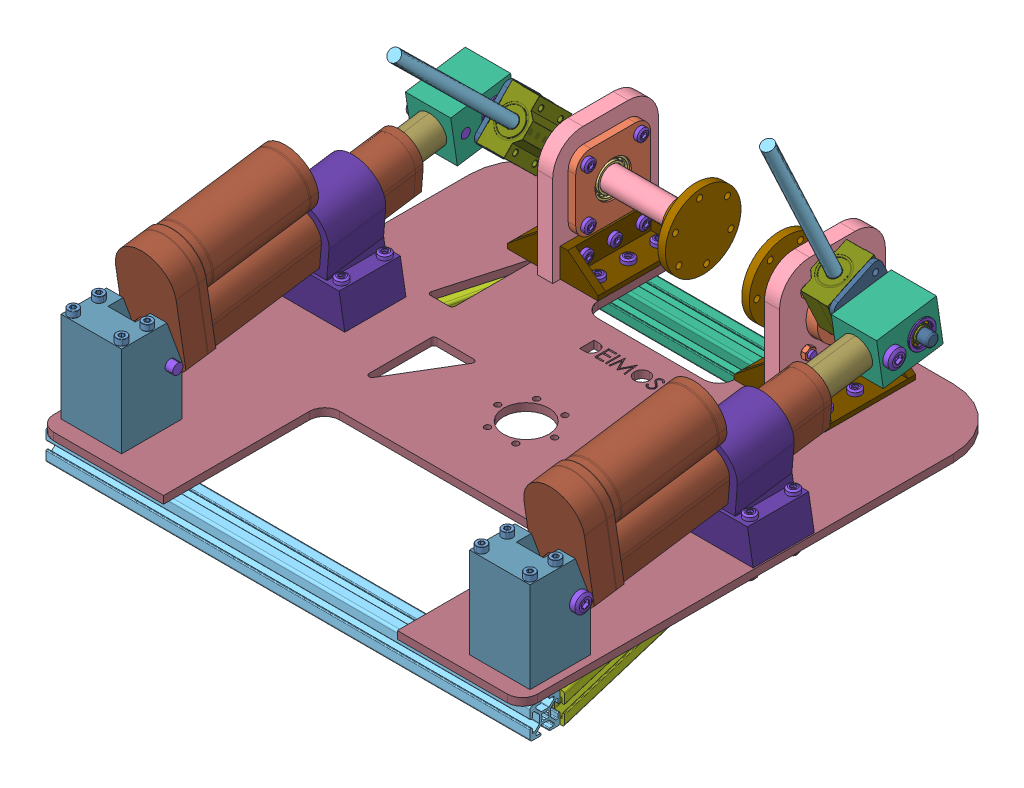
SolidWorks assembly Arm_base_2025_Final, configuration Default. Lengths in mm. (continued)
Mates (geometry in assembly coordinates): (continued)
- Distance14: distance = 6 mm anti-aligned: plane of V8_bearing and cam connection_for_v4URC 2024_V4 laser cut-2 through (396.4714 168.2112 182.1724) normal (1 0 0); plane of Connector to Linear bearing-2/V8_F688ZZ_assemblyURC 2024_V4-2/V8_F688ZZ_HousingURC 2024_V4-1 through (402.4714 162.026 159.969) normal (-1 0 0)
- Distance16: distance = 6 mm anti-aligned: plane of V8_bearing and cam connection_for_v4URC 2024_V4 laser cut-1 through (170.6714 137.31 173.1714) normal (-1 0 0); plane of Connector to Linear bearing-1/V8_F688ZZ_assemblyURC 2024_V4-1/V8_F688ZZ_HousingURC 2024_V4-1 through (164.6714 160.303 171.5672) normal (1 0 0)
- Coincident76: coincident anti-aligned: plane of base bearing assambly-1/base shaft bearing housing-1 through (213.5714 172.6403 148.5796) normal (-1 0 0); plane of V8_bearing holder holderURC 2024_V4-1 through (213.5714 172.6403 113.5796) normal (1 0 0)
- Concentric84: concentric anti-aligned: cylinder of base bearing assambly-1/base shaft bearing housing-1 through (208.5714 155.1403 166.0796) axis (1 0 0) radius 2; cylinder of V8_bearing holder holderURC 2024_V4-1 through (213.5714 155.1403 166.0796) axis (-1 0 0) radius 2
- Concentric91: concentric aligned: cylinder of LA_back holder-2 through (402.5714 180.6403 419.5796) axis (0 -1 0) radius 2; cylinder of Screw_DIN_912_M4x70_A2.step-1 through (402.5714 102.6403 419.5796) axis (0 -1 0) radius 2
- Coincident83: coincident anti-aligned: plane of LA_back holder-2 through (418.5714 152.6403 403.5796) normal (0 1 0); plane of Screw_DIN_912_M4x70_A2.step-1 through (402.5714 152.6403 419.5796) normal (0 -1 0)
- Concentric92: concentric aligned: cylinder of LA_back holder-2 through (434.5714 180.6403 419.5796) axis (0 -1 0) radius 2; cylinder of Screw_DIN_912_M4x70_A2.step-2 through (434.5714 102.6403 419.5796) axis (0 -1 0) radius 2
- Coincident84: coincident anti-aligned: plane of LA_back holder-2 through (418.5714 152.6403 403.5796) normal (0 1 0); plane of Screw_DIN_912_M4x70_A2.step-2 through (434.5714 152.6403 419.5796) normal (0 -1 0)
- Concentric93: concentric aligned: cylinder of LA_back holder-2 through (434.5714 180.6403 402.6026) axis (0 -1 0) radius 2; cylinder of Screw_DIN_912_M4x70_A2.step-4 through (434.5714 102.6403 402.6026) axis (0 -1 0) radius 2
- Coincident85: coincident anti-aligned: plane of LA_back holder-2 through (418.5714 152.6403 403.5796) normal (0 1 0); plane of Screw_DIN_912_M4x70_A2.step-4 through (434.5714 152.6403 402.6026) normal (0 -1 0)
- Concentric94: concentric aligned: cylinder of LA_back holder-2 through (402.5714 180.6403 402.6026) axis (0 -1 0) radius 2; cylinder of Screw_DIN_912_M4x70_A2.step-6 through (402.5714 102.6403 402.6026) axis (0 -1 0) radius 2
- Coincident86: coincident anti-aligned: plane of LA_back holder-2 through (418.5714 152.6403 403.5796) normal (0 1 0); plane of Screw_DIN_912_M4x70_A2.step-6 through (402.5714 152.6403 402.6026) normal (0 -1 0)
- Concentric95: concentric aligned: cylinder of LA_back holder-1 through (164.5714 180.6403 419.5796) axis (0 -1 0) radius 2; cylinder of Screw_DIN_912_M4x70_A2.step-8 through (164.5714 102.6403 419.5796) axis (0 -1 0) radius 2
- Coincident87: coincident anti-aligned: plane of LA_back holder-1 through (148.5714 152.6403 403.5796) normal (0 1 0); plane of Screw_DIN_912_M4x70_A2.step-8 through (164.5714 152.6403 419.5796) normal (0 -1 0)
- Concentric96: concentric aligned: cylinder of LA_back holder-1 through (164.5714 180.6403 402.6026) axis (0 -1 0) radius 2; cylinder of Screw_DIN_912_M4x70_A2.step-10 through (164.5714 102.6403 402.6026) axis (0 -1 0) radius 2
- Coincident88: coincident anti-aligned: plane of LA_back holder-1 through (148.5714 152.6403 403.5796) normal (0 1 0); plane of Screw_DIN_912_M4x70_A2.step-10 through (164.5714 152.6403 402.6026) normal (0 -1 0)
- Concentric97: concentric aligned: cylinder of LA_back holder-1 through (132.5714 180.6403 419.5796) axis (0 -1 0) radius 2; cylinder of Screw_DIN_912_M4x70_A2.step-12 through (132.5714 102.6403 419.5796) axis (0 -1 0) radius 2
- Coincident89: coincident anti-aligned: plane of LA_back holder-1 through (148.5714 152.6403 403.5796) normal (0 1 0); plane of Screw_DIN_912_M4x70_A2.step-12 through (132.5714 152.6403 419.5796) normal (0 -1 0)
- Concentric98: concentric aligned: cylinder of LA_back holder-1 through (132.5714 180.6403 402.6026) axis (0 -1 0) radius 2; cylinder of Screw_DIN_912_M4x70_A2.step-14 through (132.5714 102.6403 402.6026) axis (0 -1 0) radius 2
- Coincident90: coincident anti-aligned: plane of LA_back holder-1 through (148.5714 152.6403 403.5796) normal (0 1 0); plane of Screw_DIN_912_M4x70_A2.step-14 through (132.5714 152.6403 402.6026) normal (0 -1 0)
- Concentric99: concentric anti-aligned: cylinder of V8_base plate for LAURC 2024_V4-1 through (402.5714 82.6403 419.5796) axis (0 1 0) radius 2; cylinder of hex nut style 1 gradeab_iso-8 through (402.5714 87.6403 419.5796) axis (0 -1 0) radius 1.65
- Coincident91: coincident anti-aligned: plane of V8_base plate for LAURC 2024_V4-1 through (283.5714 87.6403 412.2334) normal (0 -1 0); plane of hex nut style 1 gradeab_iso-8 through (395.5728 87.6403 419.4444) normal (0 1 0)
- Concentric100: concentric anti-aligned: cylinder of V8_base plate for LAURC 2024_V4-1 through (434.5714 82.6403 419.5796) axis (0 1 0) radius 2; cylinder of hex nut style 1 gradeab_iso-9 through (434.5714 87.6403 419.5796) axis (0 -1 0) radius 1.65
- Coincident92: coincident anti-aligned: plane of V8_base plate for LAURC 2024_V4-1 through (283.5714 87.6403 412.2334) normal (0 -1 0); plane of hex nut style 1 gradeab_iso-9 through (427.6727 87.6403 420.7658) normal (0 1 0)
- Concentric101: concentric aligned: circle of Screw_DIN_912_M4x70_A2.step-4; cylinder of hex nut style 1 gradeab_iso-11 through (434.5714 87.6403 402.6026) axis (0 -1 0) radius 1.65
- Coincident93: coincident anti-aligned: plane of V8_base plate for LAURC 2024_V4-1 through (283.5714 87.6403 412.2334) normal (0 -1 0); plane of hex nut style 1 gradeab_iso-11 through (430.6304 87.6403 408.3878) normal (0 1 0)
- Concentric102: concentric aligned: cylinder of Screw_DIN_912_M4x70_A2.step-6; cylinder of hex nut style 1 gradeab_iso-14 through (402.5714 87.6403 402.6026) axis (0 -1 0) radius 1.65
- Coincident94: coincident anti-aligned: plane of V8_base plate for LAURC 2024_V4-1 through (283.5714 87.6403 412.2334) normal (0 -1 0); plane of hex nut style 1 gradeab_iso-14 through (398.6304 87.6403 408.3878) normal (0 1 0)
- Concentric103: concentric anti-aligned: cylinder of V8_base plate for LAURC 2024_V4-1; cylinder of hex nut style 1 gradeab_iso-16 through (164.5714 87.6403 419.5796) axis (0 -1 0) radius 1.65
- Coincident95: coincident anti-aligned: plane of V8_base plate for LAURC 2024_V4-1 through (283.5714 87.6403 412.2334) normal (0 -1 0); plane of hex nut style 1 gradeab_iso-16 through (160.0326 87.6403 424.9087) normal (0 1 0)
- Concentric104: concentric aligned: cylinder of Screw_DIN_912_M4x70_A2.step-10; cylinder of hex nut style 1 gradeab_iso-18 through (164.5714 87.6403 402.6026) axis (0 -1 0) radius 1.65
- Coincident96: coincident anti-aligned: plane of V8_base plate for LAURC 2024_V4-1 through (283.5714 87.6403 412.2334) normal (0 -1 0); plane of hex nut style 1 gradeab_iso-18 through (160.6304 87.6403 408.3878) normal (0 1 0)
- Concentric105: concentric aligned: cylinder of Screw_DIN_912_M4x70_A2.step-12; cylinder of hex nut style 1 gradeab_iso-20 through (132.5714 87.6403 419.5796) axis (0 -1 0) radius 1.65
- Coincident97: coincident anti-aligned: plane of V8_base plate for LAURC 2024_V4-1 through (283.5714 87.6403 412.2334) normal (0 -1 0); plane of hex nut style 1 gradeab_iso-20 through (128.6304 87.6403 425.3648) normal (0 1 0)
- Concentric106: concentric aligned: cylinder of Screw_DIN_912_M4x70_A2.step-14; cylinder of hex nut style 1 gradeab_iso-22 through (132.5714 87.6403 402.6026) axis (0 -1 0) radius 1.65
- Coincident98: coincident anti-aligned: plane of V8_base plate for LAURC 2024_V4-1 through (283.5714 87.6403 412.2334) normal (0 -1 0); plane of hex nut style 1 gradeab_iso-22 through (128.6304 87.6403 408.3878) normal (0 1 0)
- Concentric107: concentric aligned: unknown of linnear rod coupler-2; unknown of lock_nut_for coupler-2
- Concentric108: concentric aligned: cylinder of lock_nut_for coupler-2; cylinder of base bearing assambly-2/base shaft bearing housing-1 through (370.5714 137.6403 148.5796) axis (1 0 0) radius 8
- Coincident100: coincident anti-aligned: plane of V8_base plate for LAURC 2024_V4-1 through (283.5714 92.6403 412.2334) normal (0 1 0); plane of linear_acutator_holder-1 through (394.6971 92.6403 239.7077) normal (0 -1 0)
- Tangent2: tangent: cylinder of linnear rod coupler-2 through (388.2714 137.6403 148.5796) axis (-1 0 0) radius 6; unknown of linear guid rod-2
- Tangent3: tangent: cylinder of linnear rod coupler-1 through (178.8714 137.6403 148.5796) axis (1 0 0) radius 6; unknown of linear guid rod-1
- Concentric109: concentric anti-aligned: cylinder of linnear rod coupler-1 through (178.8714 137.6403 148.5796) axis (1 0 0) radius 6; cylinder of base bearing assambly-1/base shaft bearing housing-1 through (196.5714 137.6403 148.5796) axis (-1 0 0) radius 8
- Concentric110: concentric anti-aligned: cylinder of base bearing assambly-2/base shaft bearing housing-1 through (370.5714 137.6403 148.5796) axis (1 0 0) radius 8; cylinder of V8_shaftURC 2024_V4 real part-1 through (333.5714 137.6403 148.5796) axis (-1 0 0) radius 7.5
- Concentric111: concentric anti-aligned: cylinder of base bearing assambly-1/base shaft bearing housing-1 through (196.5714 137.6403 148.5796) axis (-1 0 0) radius 8; cylinder of V8_shaftURC 2024_V4-1 through (273.0714 137.6403 148.5796) axis (1 0 0) radius 7.5
- Coincident102: coincident aligned: plane of V8_bearing holder holderURC 2024_V4-1 through (203.5714 172.6403 113.5796) normal (0 0 -1); plane of V8_bearing holder holderURC 2024_V4-2 through (363.5714 172.6403 113.5796) normal (0 0 -1)
- Coincident105: coincident aligned: plane of linnear rod coupler-1 through (170.8714 137.6403 148.5796) normal (-1 0 0); plane of V8_shaftURC 2024_V4-1 through (170.8714 137.6403 148.5796) normal (-1 0 0)
- Coincident106: coincident anti-aligned: plane of V8_base plate for LAURC 2024_V4-1 through (283.5714 87.6403 412.2334) normal (0 -1 0); plane of 20 20 aluminium extrusion T slot-1 through (443.5714 87.6403 427.0796) normal (0 1 0)
- Coincident107: coincident aligned: plane of V8_base plate for LAURC 2024_V4-1 through (443.5714 92.6403 412.2334) normal (1 0 0); plane of 20 20 aluminium extrusion T slot-1 through (443.5714 74.5023 409.0876) normal (1 0 0)
- Distance17: distance = 5 mm aligned: plane of 20 20 aluminium extrusion T slot-1 through (443.5714 69.1403 428.5796) normal (0 0 1); plane of V8_base plate for LAURC 2024_V4-1 through (283.5714 92.6403 433.5796) normal (0 0 1)
- Coincident108: coincident anti-aligned: plane of V8_base plate for LAURC 2024_V4-1 through (283.5714 87.6403 412.2334) normal (0 -1 0); plane of 20 20 aluminium extrusion T slot 200 mm-1 through (383.5714 87.6403 157.0796) normal (0 1 0)
- Parallel18: parallel aligned: plane of V8_base plate for LAURC 2024_V4-1 through (443.5714 92.6403 412.2334) normal (1 0 0); plane of 20 20 aluminium extrusion T slot 200 mm-1 through (383.5714 74.5023 139.0876) normal (1 0 0)
- Coincident109: coincident anti-aligned: plane of V8_base plate for LAURC 2024_V4-1 through (283.5714 87.6403 412.2334) normal (0 -1 0); plane of 20 20 aluminium extrusion T slot at angle-1 through (383.9984 87.6403 154.2734) normal (0 1 0)
- Distance18: distance = 60 mm aligned: plane of V8_base plate for LAURC 2024_V4-1 through (443.5714 92.6403 412.2334) normal (1 0 0); plane of 20 20 aluminium extrusion T slot 200 mm-1 through (383.5714 74.5023 139.0876) normal (1 0 0)
- Coincident111: coincident anti-aligned: plane of 20 20 aluminium extrusion T slot 200 mm-1 through (383.5714 69.1403 158.5796) normal (0 0 1); plane of 20 20 aluminium extrusion T slot at angle-1 through (386.5714 87.6403 158.5796) normal (0 0 -1)
- Distance20: distance = 30 mm aligned: plane of V8_base plate for LAURC 2024_V4-1 through (283.5714 92.6403 108.5796) normal (0 0 -1); plane of 20 20 aluminium extrusion T slot 200 mm-1 through (383.5714 86.1403 138.5796) normal (0 0 -1)
- Coincident113: coincident anti-aligned: plane of 20 20 aluminium extrusion T slot 200 mm-1 through (383.5714 69.1403 158.5796) normal (0 0 1); plane of 20 20 aluminium extrusion T slot at angle-2 through (201.1363 67.6403 158.5796) normal (0 0 -1)
- Parallel19: parallel anti-aligned: plane of 20 20 aluminium extrusion T slot-1 through (443.5714 74.5023 408.5796) normal (0 0 -1); plane of 20 20 aluminium extrusion T slot at angle-2 through (141.3123 67.6403 408.5333) normal (0 0 1)
- Coincident115: coincident anti-aligned: plane of V8_base plate for LAURC 2024_V4-1 through (283.5714 87.6403 412.2334) normal (0 -1 0); plane of 20 20 aluminium extrusion T slot at angle-2 through (122.2062 87.6403 408.8825) normal (0 1 0)
- Distance21: distance = 3 mm aligned: line of 20 20 aluminium extrusion T slot at angle-2 through (180.5714 69.1403 158.5796) axis (0 1 0); line of 20 20 aluminium extrusion T slot 200 mm-1 through (183.5714 69.1403 158.5796) axis (0 1 0)
- Lock1: lock: 
- Concentric112: concentric anti-aligned: cylinder of l bracket_arm base flang-1 through (378.5714 90.6403 168.5796) axis (0 1 0) radius 2; cylinder of hexalobular socket pan head_iso-2 through (378.5714 83.6403 168.5796) axis (0 -1 0) radius 2.35
- Coincident116: coincident anti-aligned: plane of l bracket_arm base flang-1 through (388.5714 95.6403 178.5796) normal (0 1 0); plane of hexalobular socket pan head_iso-2 through (380.9214 95.6403 168.5796) normal (0 -1 0)
- Concentric113: concentric anti-aligned: cylinder of l bracket_arm base flang-1 through (378.5714 90.6403 148.5796) axis (0 1 0) radius 2; cylinder of hexalobular socket pan head_iso-3 through (378.5714 83.6403 148.5796) axis (0 -1 0) radius 2.35
- Coincident117: coincident anti-aligned: plane of l bracket_arm base flang-1 through (388.5714 95.6403 178.5796) normal (0 1 0); plane of hexalobular socket pan head_iso-3 through (380.9214 95.6403 148.5796) normal (0 -1 0)
- Concentric114: concentric anti-aligned: cylinder of l bracket_arm base flang-1 through (378.5714 90.6403 128.5796) axis (0 1 0) radius 2; cylinder of hexalobular socket pan head_iso-4 through (378.5714 83.6403 128.5796) axis (0 -1 0) radius 2.35
- Coincident118: coincident anti-aligned: plane of l bracket_arm base flang-1 through (388.5714 95.6403 178.5796) normal (0 1 0); plane of hexalobular socket pan head_iso-4 through (380.9214 95.6403 128.5796) normal (0 -1 0)
- Concentric115: concentric anti-aligned: cylinder of l bracket_arm base flang-2 through (338.5714 90.6403 168.5796) axis (0 1 0) radius 2; cylinder of hexalobular socket pan head_iso-5 through (338.5714 83.6403 168.5796) axis (0 -1 0) radius 2.35
- Coincident119: coincident anti-aligned: plane of l bracket_arm base flang-2 through (328.5714 95.6403 118.5796) normal (0 1 0); plane of hexalobular socket pan head_iso-5 through (340.9214 95.6403 168.5796) normal (0 -1 0)
- Concentric116: concentric anti-aligned: cylinder of l bracket_arm base flang-2 through (338.5714 90.6403 148.5796) axis (0 1 0) radius 2; cylinder of hexalobular socket pan head_iso-6 through (338.5714 83.6403 148.5796) axis (0 -1 0) radius 2.35
- Coincident120: coincident anti-aligned: plane of l bracket_arm base flang-2 through (328.5714 95.6403 118.5796) normal (0 1 0); plane of hexalobular socket pan head_iso-6 through (340.9214 95.6403 148.5796) normal (0 -1 0)
- Concentric117: concentric anti-aligned: cylinder of l bracket_arm base flang-2 through (338.5714 90.6403 128.5796) axis (0 1 0) radius 2; cylinder of hexalobular socket pan head_iso-7 through (338.5714 83.6403 128.5796) axis (0 -1 0) radius 2.35
- Coincident121: coincident anti-aligned: plane of l bracket_arm base flang-2 through (328.5714 95.6403 118.5796) normal (0 1 0); plane of hexalobular socket pan head_iso-7 through (340.9214 95.6403 128.5796) normal (0 -1 0)
- Concentric118: concentric anti-aligned: cylinder of l bracket_arm base flang-4 through (228.5714 90.6403 128.5796) axis (0 1 0) radius 2; cylinder of hexalobular socket pan head_iso-8 through (228.5714 83.6403 128.5796) axis (0 -1 0) radius 2.35
- Coincident122: coincident anti-aligned: plane of l bracket_arm base flang-4 through (238.5714 95.6403 178.5796) normal (0 1 0); plane of hexalobular socket pan head_iso-8 through (230.9214 95.6403 128.5796) normal (0 -1 0)
- Concentric119: concentric anti-aligned: cylinder of l bracket_arm base flang-4 through (228.5714 90.6403 148.5796) axis (0 1 0) radius 2; cylinder of hexalobular socket pan head_iso-9 through (228.5714 83.6403 148.5796) axis (0 -1 0) radius 2.35
- Coincident123: coincident anti-aligned: plane of l bracket_arm base flang-4 through (238.5714 95.6403 178.5796) normal (0 1 0); plane of hexalobular socket pan head_iso-9 through (230.9214 95.6403 148.5796) normal (0 -1 0)
- Concentric120: concentric anti-aligned: cylinder of l bracket_arm base flang-4 through (228.5714 90.6403 168.5796) axis (0 1 0) radius 2; cylinder of hexalobular socket pan head_iso-10 through (228.5714 83.6403 168.5796) axis (0 -1 0) radius 2.35
- Coincident124: coincident anti-aligned: plane of l bracket_arm base flang-4 through (238.5714 95.6403 178.5796) normal (0 1 0); plane of hexalobular socket pan head_iso-10 through (230.9214 95.6403 168.5796) normal (0 -1 0)
- Concentric121: concentric anti-aligned: cylinder of l bracket_arm base flang-3 through (188.5714 90.6403 128.5796) axis (0 1 0) radius 2; cylinder of hexalobular socket pan head_iso-11 through (188.5714 83.6403 128.5796) axis (0 -1 0) radius 2.35
- Coincident125: coincident anti-aligned: plane of l bracket_arm base flang-3 through (178.5714 95.6403 118.5796) normal (0 1 0); plane of hexalobular socket pan head_iso-11 through (190.9214 95.6403 128.5796) normal (0 -1 0)
- Concentric122: concentric anti-aligned: cylinder of l bracket_arm base flang-3 through (188.5714 90.6403 148.5796) axis (0 1 0) radius 2; cylinder of hexalobular socket pan head_iso-12 through (188.5714 83.6403 148.5796) axis (0 -1 0) radius 2.35
- Coincident126: coincident anti-aligned: plane of l bracket_arm base flang-3 through (178.5714 95.6403 118.5796) normal (0 1 0); plane of hexalobular socket pan head_iso-12 through (190.9214 95.6403 148.5796) normal (0 -1 0)
- Concentric123: concentric anti-aligned: cylinder of l bracket_arm base flang-3 through (188.5714 90.6403 168.5796) axis (0 1 0) radius 2; cylinder of hexalobular socket pan head_iso-13 through (188.5714 83.6403 168.5796) axis (0 -1 0) radius 2.35
- Coincident127: coincident anti-aligned: plane of l bracket_arm base flang-3 through (178.5714 95.6403 118.5796) normal (0 1 0); plane of hexalobular socket pan head_iso-13 through (190.9214 95.6403 168.5796) normal (0 -1 0)
- Concentric125: concentric anti-aligned: cylinder of l bracket_arm base flang-2 through (353.5714 103.6403 129.5796) axis (-1 0 0) radius 1.6729; cylinder of hexalobular socket pan head_iso-16 through (373.5714 103.6403 129.5796) axis (1 0 0) radius 2.35
- Coincident129: coincident anti-aligned: plane of l bracket_arm base flang-2 through (348.5714 111.6403 118.5796) normal (-1 0 0); plane of hexalobular socket pan head_iso-16 through (348.5714 105.9903 129.5796) normal (1 0 0)
- Concentric126: concentric anti-aligned: cylinder of l bracket_arm base flang-2 through (353.5714 103.6403 148.5796) axis (-1 0 0) radius 1.6729; cylinder of hexalobular socket pan head_iso-17 through (373.5714 103.6403 148.5796) axis (1 0 0) radius 2.35
- Coincident130: coincident anti-aligned: plane of l bracket_arm base flang-2 through (348.5714 111.6403 118.5796) normal (-1 0 0); plane of hexalobular socket pan head_iso-17 through (348.5714 105.9903 148.5796) normal (1 0 0)
- Concentric127: concentric anti-aligned: cylinder of l bracket_arm base flang-2 through (353.5714 103.6403 167.5796) axis (-1 0 0) radius 1.6729; cylinder of hexalobular socket pan head_iso-18 through (373.5714 103.6403 167.5796) axis (1 0 0) radius 2.35
- Coincident131: coincident anti-aligned: plane of l bracket_arm base flang-2 through (348.5714 111.6403 118.5796) normal (-1 0 0); plane of hexalobular socket pan head_iso-18 through (348.5714 105.9903 167.5796) normal (1 0 0)
- Concentric128: concentric anti-aligned: cylinder of l bracket_arm base flang-4 through (213.5714 103.6403 167.5796) axis (1 0 0) radius 1.6729; cylinder of hexalobular socket pan head_iso-19 through (193.5714 103.6403 167.5796) axis (-1 0 0) radius 2.35
- Coincident132: coincident anti-aligned: plane of l bracket_arm base flang-4 through (218.5714 111.6403 178.5796) normal (1 0 0); plane of hexalobular socket pan head_iso-19 through (218.5714 101.2903 167.5796) normal (-1 0 0)
- Concentric129: concentric anti-aligned: cylinder of l bracket_arm base flang-4 through (213.5714 103.6403 148.5796) axis (1 0 0) radius 1.6729; cylinder of hexalobular socket pan head_iso-20 through (193.5714 103.6403 148.5796) axis (-1 0 0) radius 2.35
- Coincident133: coincident anti-aligned: plane of l bracket_arm base flang-4 through (218.5714 111.6403 178.5796) normal (1 0 0); plane of hexalobular socket pan head_iso-20 through (218.5714 101.2903 148.5796) normal (-1 0 0)
- Concentric130: concentric anti-aligned: cylinder of l bracket_arm base flang-4 through (213.5714 103.6403 129.5796) axis (1 0 0) radius 1.6729; cylinder of hexalobular socket pan head_iso-21 through (193.5714 103.6403 129.5796) axis (-1 0 0) radius 2.35
- Coincident134: coincident anti-aligned: plane of l bracket_arm base flang-4 through (218.5714 111.6403 178.5796) normal (1 0 0); plane of hexalobular socket pan head_iso-21 through (218.5714 101.2903 129.5796) normal (-1 0 0)
- Concentric131: concentric anti-aligned: cylinder of base bearing assambly-2/base shaft bearing housing-1 through (358.5714 155.1403 131.0796) axis (-1 0 0) radius 2; cylinder of hexalobular socket pan head_iso-23 through (368.5714 155.1403 131.0796) axis (1 0 0) radius 2.35
- Coincident135: coincident anti-aligned: plane of base bearing assambly-2/base shaft bearing housing-1 through (348.5714 149.6403 148.5796) normal (-1 0 0); plane of hexalobular socket pan head_iso-23 through (348.5714 157.4903 131.0796) normal (1 0 0)
- Concentric132: concentric anti-aligned: cylinder of base bearing assambly-2/base shaft bearing housing-1 through (358.5714 155.1403 166.0796) axis (-1 0 0) radius 2; cylinder of hexalobular socket pan head_iso-24 through (368.5714 155.1403 166.0796) axis (1 0 0) radius 2.35
- Coincident136: coincident anti-aligned: plane of base bearing assambly-2/base shaft bearing housing-1 through (348.5714 149.6403 148.5796) normal (-1 0 0); plane of hexalobular socket pan head_iso-24 through (348.5714 157.4903 166.0796) normal (1 0 0)
- Concentric133: concentric anti-aligned: cylinder of base bearing assambly-2/base shaft bearing housing-1 through (358.5714 120.1403 131.0796) axis (-1 0 0) radius 2; cylinder of hexalobular socket pan head_iso-25 through (368.5714 120.1403 131.0796) axis (1 0 0) radius 2.35
- Coincident137: coincident anti-aligned: plane of base bearing assambly-2/base shaft bearing housing-1 through (348.5714 149.6403 148.5796) normal (-1 0 0); plane of hexalobular socket pan head_iso-25 through (348.5714 122.4903 131.0796) normal (1 0 0)
- Concentric134: concentric anti-aligned: cylinder of base bearing assambly-2/base shaft bearing housing-1 through (358.5714 120.1403 166.0796) axis (-1 0 0) radius 2; cylinder of hexalobular socket pan head_iso-26 through (368.5714 120.1403 166.0796) axis (1 0 0) radius 2.35
- Coincident138: coincident anti-aligned: plane of base bearing assambly-2/base shaft bearing housing-1 through (348.5714 149.6403 148.5796) normal (-1 0 0); plane of hexalobular socket pan head_iso-26 through (348.5714 122.4903 166.0796) normal (1 0 0)
- Concentric1351: concentric anti-aligned: cylinder of base bearing assambly-1/base shaft bearing housing-1 through (208.5714 120.1403 131.0796) axis (1 0 0) radius 2; cylinder of hexalobular socket pan head_iso-27 through (198.5714 120.1403 131.0796) axis (-1 0 0) radius 2.35
- Coincident1391: coincident anti-aligned: plane of base bearing assambly-1/base shaft bearing housing-1 through (218.5714 149.6403 148.5796) normal (1 0 0); plane of hexalobular socket pan head_iso-27 through (218.5714 117.7903 131.0796) normal (-1 0 0)
- Concentric136: concentric anti-aligned: cylinder of base bearing assambly-1/base shaft bearing housing-1 through (208.5714 155.1403 131.0796) axis (1 0 0) radius 2; cylinder of hexalobular socket pan head_iso-28 through (198.5714 155.1403 131.0796) axis (-1 0 0) radius 2.35
- Coincident140: coincident anti-aligned: plane of base bearing assambly-1/base shaft bearing housing-1 through (218.5714 149.6403 148.5796) normal (1 0 0); plane of hexalobular socket pan head_iso-28 through (218.5714 152.7903 131.0796) normal (-1 0 0)
- Concentric137: concentric anti-aligned: cylinder of base bearing assambly-1/base shaft bearing housing-1 through (208.5714 155.1403 166.0796) axis (1 0 0) radius 2; cylinder of hexalobular socket pan head_iso-29 through (198.5714 155.1403 166.0796) axis (-1 0 0) radius 2.35
- Coincident141: coincident anti-aligned: plane of base bearing assambly-1/base shaft bearing housing-1 through (218.5714 149.6403 148.5796) normal (1 0 0); plane of hexalobular socket pan head_iso-29 through (218.5714 152.7903 166.0796) normal (-1 0 0)
- Concentric138: concentric anti-aligned: cylinder of base bearing assambly-1/base shaft bearing housing-1 through (208.5714 120.1403 166.0796) axis (1 0 0) radius 2; cylinder of hexalobular socket pan head_iso-30 through (198.5714 120.1403 166.0796) axis (-1 0 0) radius 2.35
- Coincident142: coincident anti-aligned: plane of base bearing assambly-1/base shaft bearing housing-1 through (218.5714 149.6403 148.5796) normal (1 0 0); plane of hexalobular socket pan head_iso-30 through (218.5714 117.7903 166.0796) normal (-1 0 0)
- Concentric139: concentric anti-aligned: cylinder of linear_acutator_holder-1 through (437.6971 82.0703 277.3153) axis (0 1 0) radius 2; cylinder of hexalobular socket pan head_iso-32 through (437.6971 83.0703 277.3153) axis (0 -1 0) radius 2.35
- Coincident143: coincident anti-aligned: plane of linear_acutator_holder-1 through (394.6971 118.0703 243.4855) normal (0 1 0); plane of hexalobular socket pan head_iso-32 through (440.0471 118.0703 277.3153) normal (0 -1 0)
- Concentric140: concentric anti-aligned: cylinder of linear_acutator_holder-1 through (437.6971 82.0703 248.7068) axis (0 1 0) radius 2; cylinder of hexalobular socket pan head_iso-33 through (437.6971 83.0703 248.7068) axis (0 -1 0) radius 2.35
- Coincident144: coincident anti-aligned: plane of linear_acutator_holder-1 through (394.6971 118.0703 243.4855) normal (0 1 0); plane of hexalobular socket pan head_iso-33 through (440.0471 118.0703 248.7068) normal (0 -1 0)
- Concentric141: concentric anti-aligned: cylinder of linear_acutator_holder-1 through (399.6971 82.0703 277.3153) axis (0 1 0) radius 2; cylinder of hexalobular socket pan head_iso-34 through (399.6971 83.0703 277.3153) axis (0 -1 0) radius 2.35
- Coincident145: coincident anti-aligned: plane of linear_acutator_holder-1 through (394.6971 118.0703 243.4855) normal (0 1 0); plane of hexalobular socket pan head_iso-34 through (402.0471 118.0703 277.3153) normal (0 -1 0)
- Concentric142: concentric anti-aligned: cylinder of linear_acutator_holder-1 through (399.6971 82.0703 248.7068) axis (0 1 0) radius 2; cylinder of hexalobular socket pan head_iso-35 through (399.6971 83.0703 248.7068) axis (0 -1 0) radius 2.35
- Coincident146: coincident anti-aligned: plane of linear_acutator_holder-1 through (394.6971 118.0703 243.4855) normal (0 1 0); plane of hexalobular socket pan head_iso-35 through (402.0471 118.0703 248.7068) normal (0 -1 0)
- Concentric143: concentric anti-aligned: cylinder of linear_acutator_holder-2 through (129.6971 82.0703 248.7068) axis (0 1 0) radius 2; cylinder of hexalobular socket pan head_iso-36 through (129.6971 83.0703 248.7068) axis (0 -1 0) radius 2.35
- Coincident147: coincident anti-aligned: plane of linear_acutator_holder-2 through (124.6971 118.0703 243.4855) normal (0 1 0); plane of hexalobular socket pan head_iso-36 through (132.0471 118.0703 248.7068) normal (0 -1 0)
- Concentric144: concentric anti-aligned: cylinder of linear_acutator_holder-2 through (129.6971 82.0703 277.3153) axis (0 1 0) radius 2; cylinder of hexalobular socket pan head_iso-37 through (129.6971 83.0703 277.3153) axis (0 -1 0) radius 2.35
- Coincident148: coincident anti-aligned: plane of linear_acutator_holder-2 through (124.6971 118.0703 243.4855) normal (0 1 0); plane of hexalobular socket pan head_iso-37 through (132.0471 118.0703 277.3153) normal (0 -1 0)
- Concentric145: concentric anti-aligned: cylinder of linear_acutator_holder-2 through (167.6971 82.0703 248.7068) axis (0 1 0) radius 2; cylinder of hexalobular socket pan head_iso-38 through (167.6971 83.0703 248.7068) axis (0 -1 0) radius 2.35
- Coincident149: coincident anti-aligned: plane of linear_acutator_holder-2 through (124.6971 118.0703 243.4855) normal (0 1 0); plane of hexalobular socket pan head_iso-38 through (170.0471 118.0703 248.7068) normal (0 -1 0)
- Concentric146: concentric anti-aligned: cylinder of linear_acutator_holder-2 through (167.6971 82.0703 277.3153) axis (0 1 0) radius 2; cylinder of hexalobular socket pan head_iso-39 through (167.6971 83.0703 277.3153) axis (0 -1 0) radius 2.35
- Coincident150: coincident anti-aligned: plane of linear_acutator_holder-2 through (124.6971 118.0703 243.4855) normal (0 1 0); plane of hexalobular socket pan head_iso-39 through (170.0471 118.0703 277.3153) normal (0 -1 0)
- Concentric147: concentric anti-aligned: cylinder of Connector to Linear bearing-1/V8_connectorURC 2024_V4-1 through (234.5714 157.4228 190.9544) axis (-1 0 0) radius 3; cylinder of hexalobular socket pan head_iso-41 through (163.5714 157.4228 190.9544) axis (1 0 0) radius 3.4
- Coincident151: coincident anti-aligned: plane of Connector to Linear bearing-1/V8_connectorURC 2024_V4-1 through (133.5714 176.977 161.4071) normal (-1 0 0); plane of hexalobular socket pan head_iso-41 through (133.5714 160.8228 190.9544) normal (1 0 0)
- Concentric148: concentric aligned: cylinder of Connector to Linear bearing-2/V8_connectorURC 2024_V4-1 through (504.5714 159.1459 179.3562) axis (-1 0 0) radius 3; cylinder of hexalobular socket pan head_iso-42 through (403.5714 159.1459 179.3562) axis (-1 0 0) radius 3.4
- Coincident152: coincident anti-aligned: plane of Connector to Linear bearing-2/V8_connectorURC 2024_V4-1 through (433.5714 178.7 149.8089) normal (1 0 0); plane of hexalobular socket pan head_iso-42 through (433.5714 155.7459 179.3562) normal (-1 0 0)
- Concentric149: concentric aligned: cylinder of hexalobular socket pan head_iso-17 through (373.5714 103.6403 148.5796) axis (1 0 0) radius 2.35; cylinder of hex nut style 1 gradeab_iso-24 through (346.7339 103.6403 148.5796) axis (1 0 0) radius 2
- Coincident153: coincident anti-aligned: plane of l bracket_arm base flang-1 through (368.5714 111.6403 178.5796) normal (1 0 0); plane of hex nut style 1 gradeab_iso-24 through (368.5714 97.2267 145.7749) normal (-1 0 0)
- Concentric150: concentric aligned: cylinder of hexalobular socket pan head_iso-18 through (373.5714 103.6403 167.5796) axis (1 0 0) radius 2.35; cylinder of hex nut style 1 gradeab_iso-25 through (346.7339 103.6403 167.5796) axis (1 0 0) radius 2
- Coincident154: coincident anti-aligned: plane of l bracket_arm base flang-1 through (368.5714 111.6403 178.5796) normal (1 0 0); plane of hex nut style 1 gradeab_iso-25 through (368.5714 103.6403 174.5796) normal (-1 0 0)
- Concentric151: concentric aligned: cylinder of hexalobular socket pan head_iso-16 through (373.5714 103.6403 129.5796) axis (1 0 0) radius 2.35; cylinder of hex nut style 1 gradeab_iso-26 through (346.7339 103.6403 129.5796) axis (1 0 0) radius 2
- Coincident155: coincident anti-aligned: plane of l bracket_arm base flang-1 through (368.5714 111.6403 178.5796) normal (1 0 0); plane of hex nut style 1 gradeab_iso-26 through (368.5714 103.6403 136.5796) normal (-1 0 0)
- Concentric152: concentric anti-aligned: cylinder of base bearing assambly-2/base shaft bearing housing-1 through (358.5714 120.1403 131.0796) axis (-1 0 0) radius 2; cylinder of hex nut style 1 gradeab_iso-27 through (341.7339 120.1403 131.0796) axis (1 0 0) radius 2
- Concentric153: concentric aligned: cylinder of hexalobular socket pan head_iso-23 through (368.5714 155.1403 131.0796) axis (1 0 0) radius 2.35; cylinder of hex nut style 1 gradeab_iso-28 through (341.7339 155.1403 131.0796) axis (1 0 0) radius 2
- Coincident157: coincident anti-aligned: plane of V8_bearing holder holderURC 2024_V4-2 through (363.5714 172.6403 183.5796) normal (1 0 0); plane of hex nut style 1 gradeab_iso-28 through (363.5714 150.101 135.9382) normal (-1 0 0)
- Concentric154: concentric aligned: cylinder of hexalobular socket pan head_iso-24 through (368.5714 155.1403 166.0796) axis (1 0 0) radius 2.35; cylinder of hex nut style 1 gradeab_iso-29 through (341.7339 155.1403 166.0796) axis (1 0 0) radius 2
- Coincident158: coincident anti-aligned: plane of V8_bearing holder holderURC 2024_V4-2 through (363.5714 172.6403 183.5796) normal (1 0 0); plane of hex nut style 1 gradeab_iso-29 through (363.5714 155.1403 173.0796) normal (-1 0 0)
- Concentric155: concentric aligned: cylinder of hexalobular socket pan head_iso-4 through (378.5714 83.6403 128.5796) axis (0 -1 0) radius 2.35; cylinder of hex nut style 1 gradeab_iso-30 through (378.5714 109.4778 128.5796) axis (0 -1 0) radius 2
- Coincident159: coincident anti-aligned: plane of V8_base plate for LAURC 2024_V4-1 through (283.5714 87.6403 412.2334) normal (0 -1 0); plane of hex nut style 1 gradeab_iso-30 through (371.5714 87.6403 128.5796) normal (0 1 0)
- Concentric156: concentric aligned: cylinder of hexalobular socket pan head_iso-7 through (338.5714 83.6403 128.5796) axis (0 -1 0) radius 2.35; cylinder of hex nut style 1 gradeab_iso-31 through (338.5714 109.4778 128.5796) axis (0 -1 0) radius 2
- Coincident160: coincident anti-aligned: plane of V8_base plate for LAURC 2024_V4-1 through (283.5714 87.6403 412.2334) normal (0 -1 0); plane of hex nut style 1 gradeab_iso-31 through (331.5714 87.6403 128.5796) normal (0 1 0)
- Concentric157: concentric aligned: cylinder of hexalobular socket pan head_iso-5 through (338.5714 83.6403 168.5796) axis (0 -1 0) radius 2.35; cylinder of hex nut style 1 gradeab_iso-32 through (338.5714 109.4778 168.5796) axis (0 -1 0) radius 2
- Coincident161: coincident anti-aligned: plane of V8_base plate for LAURC 2024_V4-1 through (283.5714 87.6403 412.2334) normal (0 -1 0); plane of hex nut style 1 gradeab_iso-32 through (331.5714 87.6403 168.5796) normal (0 1 0)
- Coincident163: coincident anti-aligned: plane of V8_bearing holder holderURC 2024_V4-2 through (363.5714 172.6403 183.5796) normal (1 0 0); plane of hex nut style 1 gradeab_iso-27 through (363.5714 120.1403 138.0796) normal (-1 0 0)
- Concentric158: concentric aligned: cylinder of hexalobular socket pan head_iso-26 through (368.5714 120.1403 166.0796) axis (1 0 0) radius 2.35; cylinder of hex nut style 1 gradeab_iso-34 through (341.7339 120.1403 166.0796) axis (1 0 0) radius 2
- Coincident164: coincident anti-aligned: plane of V8_bearing holder holderURC 2024_V4-2 through (363.5714 172.6403 183.5796) normal (1 0 0); plane of hex nut style 1 gradeab_iso-34 through (363.5714 120.1403 173.0796) normal (-1 0 0)
- Concentric159: concentric aligned: cylinder of V8_bearing holder holderURC 2024_V4-1 through (213.5714 155.1403 131.0796) axis (-1 0 0) radius 2; cylinder of hex nut style 1 gradeab_iso-35 through (225.409 155.1403 131.0796) axis (-1 0 0) radius 2
- Coincident165: coincident anti-aligned: plane of V8_bearing holder holderURC 2024_V4-1 through (203.5714 172.6403 113.5796) normal (-1 0 0); plane of hex nut style 1 gradeab_iso-35 through (203.5714 155.1403 124.0796) normal (1 0 0)
- Concentric160: concentric aligned: cylinder of V8_bearing holder holderURC 2024_V4-1 through (213.5714 120.1403 131.0796) axis (-1 0 0) radius 2; cylinder of hex nut style 1 gradeab_iso-36 through (225.409 120.1403 131.0796) axis (-1 0 0) radius 2
- Coincident166: coincident anti-aligned: plane of V8_bearing holder holderURC 2024_V4-1 through (203.5714 172.6403 113.5796) normal (-1 0 0); plane of hex nut style 1 gradeab_iso-36 through (203.5714 120.1403 124.0796) normal (1 0 0)
- Concentric161: concentric aligned: cylinder of V8_bearing holder holderURC 2024_V4-1 through (213.5714 155.1403 166.0796) axis (-1 0 0) radius 2; cylinder of hex nut style 1 gradeab_iso-37 through (225.409 155.1403 166.0796) axis (-1 0 0) radius 2
- Coincident167: coincident anti-aligned: plane of V8_bearing holder holderURC 2024_V4-1 through (203.5714 172.6403 113.5796) normal (-1 0 0); plane of hex nut style 1 gradeab_iso-37 through (203.5714 155.1403 159.0796) normal (1 0 0)
- Concentric162: concentric aligned: cylinder of V8_bearing holder holderURC 2024_V4-1 through (213.5714 120.1403 166.0796) axis (-1 0 0) radius 2; cylinder of hex nut style 1 gradeab_iso-38 through (225.409 120.1403 166.0796) axis (-1 0 0) radius 2
- Coincident168: coincident anti-aligned: plane of V8_bearing holder holderURC 2024_V4-1 through (203.5714 172.6403 113.5796) normal (-1 0 0); plane of hex nut style 1 gradeab_iso-38 through (203.5714 120.1403 159.0796) normal (1 0 0)
- Concentric163: concentric aligned: cylinder of l bracket_arm base flang-3 through (203.5714 103.6403 148.5796) axis (-1 0 0) radius 1.6729; cylinder of hex nut style 1 gradeab_iso-39 through (220.409 103.6403 148.5796) axis (-1 0 0) radius 2
- Coincident169: coincident anti-aligned: plane of l bracket_arm base flang-3 through (198.5714 111.6403 118.5796) normal (-1 0 0); plane of hex nut style 1 gradeab_iso-39 through (198.5714 103.6403 141.5796) normal (1 0 0)
- Concentric164: concentric aligned: cylinder of l bracket_arm base flang-3 through (203.5714 103.6403 167.5796) axis (-1 0 0) radius 1.6729; cylinder of hex nut style 1 gradeab_iso-40 through (220.409 103.6403 167.5796) axis (-1 0 0) radius 2
- Coincident170: coincident anti-aligned: plane of l bracket_arm base flang-3 through (198.5714 111.6403 118.5796) normal (-1 0 0); plane of hex nut style 1 gradeab_iso-40 through (198.5714 103.6403 160.5796) normal (1 0 0)
- Concentric165: concentric aligned: cylinder of l bracket_arm base flang-3 through (203.5714 103.6403 129.5796) axis (-1 0 0) radius 1.6729; cylinder of hex nut style 1 gradeab_iso-41 through (220.409 103.6403 129.5796) axis (-1 0 0) radius 2
- Coincident171: coincident anti-aligned: plane of l bracket_arm base flang-3 through (198.5714 111.6403 118.5796) normal (-1 0 0); plane of hex nut style 1 gradeab_iso-41 through (198.5714 103.6403 122.5796) normal (1 0 0)
- Concentric166: concentric aligned: cylinder of hexalobular socket pan head_iso-8 through (228.5714 83.6403 128.5796) axis (0 -1 0) radius 2.35; cylinder of hex nut style 1 gradeab_iso-42 through (228.5714 109.4778 128.5796) axis (0 -1 0) radius 2
- Coincident172: coincident anti-aligned: plane of V8_base plate for LAURC 2024_V4-1 through (283.5714 87.6403 412.2334) normal (0 -1 0); plane of hex nut style 1 gradeab_iso-42 through (221.5714 87.6403 128.5796) normal (0 1 0)
- Concentric167: concentric aligned: cylinder of hexalobular socket pan head_iso-11 through (188.5714 83.6403 128.5796) axis (0 -1 0) radius 2.35; cylinder of hex nut style 1 gradeab_iso-43 through (188.5714 109.4778 128.5796) axis (0 -1 0) radius 2
- Coincident173: coincident anti-aligned: plane of V8_base plate for LAURC 2024_V4-1 through (283.5714 87.6403 412.2334) normal (0 -1 0); plane of hex nut style 1 gradeab_iso-43 through (181.5714 87.6403 128.5796) normal (0 1 0)
- Concentric168: concentric aligned: cylinder of hexalobular socket pan head_iso-10 through (228.5714 83.6403 168.5796) axis (0 -1 0) radius 2.35; cylinder of hex nut style 1 gradeab_iso-44 through (228.5714 109.4778 168.5796) axis (0 -1 0) radius 2
- Coincident174: coincident anti-aligned: plane of V8_base plate for LAURC 2024_V4-1 through (283.5714 87.6403 412.2334) normal (0 -1 0); plane of hex nut style 1 gradeab_iso-44 through (221.5714 87.6403 168.5796) normal (0 1 0)
- Concentric169: concentric aligned: cylinder of hexalobular socket pan head_iso-37 through (129.6971 83.0703 277.3153) axis (0 -1 0) radius 2.35; cylinder of hex nut style 1 gradeab_iso-45 through (129.6971 109.4778 277.3153) axis (0 -1 0) radius 2
- Coincident175: coincident anti-aligned: plane of V8_base plate for LAURC 2024_V4-1 through (283.5714 87.6403 412.2334) normal (0 -1 0); plane of hex nut style 1 gradeab_iso-45 through (122.6971 87.6403 277.3153) normal (0 1 0)
- Concentric170: concentric aligned: cylinder of hexalobular socket pan head_iso-36 through (129.6971 83.0703 248.7068) axis (0 -1 0) radius 2.35; cylinder of hex nut style 1 gradeab_iso-46 through (129.6971 109.4778 248.7068) axis (0 -1 0) radius 2
- Coincident176: coincident anti-aligned: plane of V8_base plate for LAURC 2024_V4-1 through (283.5714 87.6403 412.2334) normal (0 -1 0); plane of hex nut style 1 gradeab_iso-46 through (122.6971 87.6403 248.7068) normal (0 1 0)
- Concentric171: concentric anti-aligned: cylinder of linear_acutator_holder-1 through (437.6971 82.0703 277.3153) axis (0 1 0) radius 2; cylinder of hex nut style 1 gradeab_iso-47 through (437.6971 109.4778 277.3153) axis (0 -1 0) radius 2
- Concentric172: concentric anti-aligned: cylinder of V8_base plate for LAURC 2024_V4-1 through (437.4458 87.6403 248.7068) axis (0 1 0) radius 2; cylinder of hex nut style 1 gradeab_iso-48 through (437.4458 109.4778 248.7068) axis (0 -1 0) radius 2
- Coincident178: coincident anti-aligned: plane of V8_base plate for LAURC 2024_V4-1 through (283.5714 87.6403 412.2334) normal (0 -1 0); plane of hex nut style 1 gradeab_iso-48 through (436.8655 87.6403 255.6827) normal (0 1 0)
- Coincident179: coincident anti-aligned: plane of V8_base plate for LAURC 2024_V4-1 through (283.5714 87.6403 412.2334) normal (0 -1 0); plane of hex nut style 1 gradeab_iso-47 through (439.9519 87.6403 283.9422) normal (0 1 0)
- Concentric173: concentric anti-aligned: cylinder of LA_back holder-1 through (196.5714 127.6403 391.4309) axis (-1 0 0) radius 3; cylinder of hexalobular socket pan head_iso-44 through (173.5714 127.6403 391.4309) axis (1 0 0) radius 3.4
- Coincident180: coincident anti-aligned: plane of LA_back holder-1 through (128.5714 92.6403 403.5796) normal (-1 0 0); plane of hexalobular socket pan head_iso-44 through (128.5714 131.0403 391.4309) normal (1 0 0)
- Concentric174: concentric aligned: cylinder of LA_back holder-2 through (466.5714 127.6403 391.4309) axis (-1 0 0) radius 3; cylinder of hexalobular socket pan head_iso-45 through (393.5714 127.6403 391.4309) axis (-1 0 0) radius 3.4
- Coincident181: coincident anti-aligned: plane of LA_back holder-2 through (438.5714 92.6403 403.5796) normal (1 0 0); plane of hexalobular socket pan head_iso-45 through (438.5714 124.2403 391.4309) normal (-1 0 0)
- Concentric1352: concentric aligned: cylinder of V8_shaftURC 2024_V4 real part-1 through (333.5714 137.6403 148.5796) axis (-1 0 0) radius 7.5; cylinder of Base Shaft connector to link 1-1 through (343.5714 137.6403 148.5796) axis (-1 0 0) radius 7.5
- Coincident1393: coincident aligned: plane of V8_base plate for LAURC 2024_V4-1 through (328.5714 97.6403 188.5796) normal (-1 0 0); plane of Base Shaft connector to link 1-1 through (328.5714 137.6403 148.5796) normal (-1 0 0)
- Concentric1353: concentric anti-aligned: unknown of V8_shaftURC 2024_V4-1; unknown of lock_nut_for coupler-3
- Coincident1394: coincident anti-aligned: plane of linnear rod coupler-1 through (170.8714 137.6403 148.5796) normal (-1 0 0); plane of lock_nut_for coupler-3 through (170.8714 137.6403 148.5796) normal (1 0 0)
- Concentric1354: concentric anti-aligned: cylinder of V8_shaftURC 2024_V4-1 through (273.0714 137.6403 148.5796) axis (1 0 0) radius 7.5; unknown of Base Shaft connector to link 1-2
- Coincident1395: coincident anti-aligned: plane of V8_shaftURC 2024_V4-1 through (273.0714 144.9751 150.1451) normal (1 0 0); plane of Base Shaft connector to link 1-2 through (273.0714 137.6403 148.5796) normal (-1 0 0)
